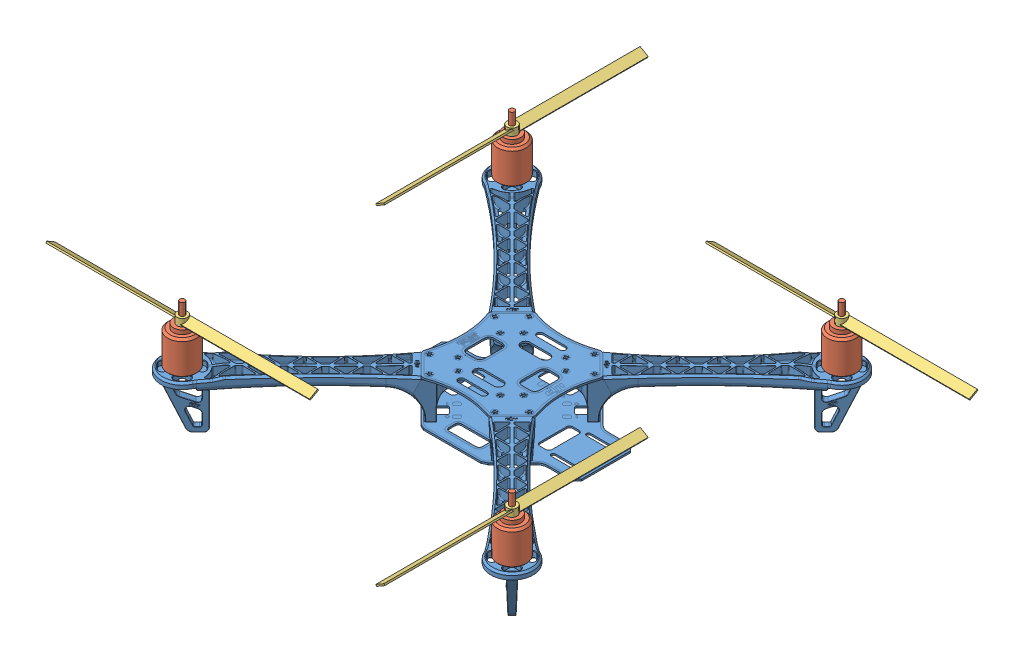
SolidWorks assembly 四旋翼机构, configuration 默认. Lengths in mm.
Overall size (571.82 108 571.82).
9 component instances, 3 part files, 26 mates.
Components (placement in the parent):
- F450 Quadcopter Frame-2: F450 Quadcopter Frame [默认] at (326.2395 -274.8713 170.1683) size (358.57 55.06 358.57)
- 旋翼电机改孔距-1: 旋翼电机改孔距 [默认] at (563.4779 -112.1783 79.5763) x (-1 0 0) z (0 0 -1) size (27.7 57 27.7)
- 螺旋桨-1: 螺旋桨 [默认] at (563.4779 -76.1783 79.5763) x (-1 0 0) z (0 0 -1) size (254 7 254)
- 旋翼电机改孔距-2: 旋翼电机改孔距 [默认] at (245.6651 -112.1783 79.5656) x (0 0 -1) z (1 0 0) size (27.7 57 27.7)
- 螺旋桨-2: 螺旋桨 [默认] at (245.6651 -76.1783 79.5656) x (0 0 -1) z (1 0 0) size (254 7 254)
- 旋翼电机改孔距-4: 旋翼电机改孔距 [默认] at (245.6757 -112.1783 -238.2473) size (27.7 57 27.7)
- 螺旋桨-4: 螺旋桨 [默认] at (245.6757 -76.1783 -238.2473) size (254 7 254)
- 旋翼电机改孔距-6: 旋翼电机改孔距 [默认] at (563.4886 -112.1783 -238.2366) x (0 0 1) z (-1 0 0) size (27.7 57 27.7)
- 螺旋桨-6: 螺旋桨 [默认] at (563.4886 -76.1783 -238.2366) x (0 0 1) z (-1 0 0) size (254 7 254)
Mates (geometry in assembly coordinates):
- 同心1: concentric: cylinder of 旋翼电机改孔距-1 through (563.4779 -57.6783 79.5763) axis (0 -1 0) radius 2.5; cylinder of 螺旋桨-1 through (563.4779 -76.1793 79.5763) axis (0 1 0) radius 2.5
- 重合1: coincident: plane of 旋翼电机改孔距-1 through (563.4779 -76.1783 79.5763) normal (0 1 0); plane of 螺旋桨-1 through (563.4779 -76.1783 79.5763) normal (0 -1 0)
- 重合2: coincident: plane of F450 Quadcopter Frame-2 through (570.6867 -112.1783 60.2935) normal (0 1 0); plane of 旋翼电机改孔距-1 through (563.4779 -112.1783 79.5763) normal (0 -1 0)
- 同心6: concentric: cylinder of F450 Quadcopter Frame-2 through (563.4779 -131.8204 79.5763) axis (0 1 0) radius 5; cylinder of 旋翼电机改孔距-1 through (563.4779 -114.6783 79.5763) axis (0 1 0) radius 2.5
- 同心9: concentric: cylinder of F450 Quadcopter Frame-2 through (554.1779 -131.8204 79.5763) axis (0 1 0) radius 1.65; cylinder of 旋翼电机改孔距-1 through (554.1779 -109.1783 79.5763) axis (0 -1 0) radius 1.35
- 同心10: concentric: cylinder of 旋翼电机改孔距-2 through (245.6651 -57.6783 79.5656) axis (0 -1 0) radius 2.5; cylinder of 螺旋桨-2 through (245.6651 -76.1793 79.5656) axis (0 1 0) radius 2.5
- 重合3: coincident: plane of 旋翼电机改孔距-2 through (245.6651 -76.1783 79.5656) normal (0 1 0); plane of 螺旋桨-2 through (245.6651 -76.1783 79.5656) normal (0 -1 0)
- 重合4: coincident: plane of F450 Quadcopter Frame-2 through (264.9479 -112.1783 86.7744) normal (0 1 0); plane of 旋翼电机改孔距-2 through (245.6651 -112.1783 79.5656) normal (0 -1 0)
- 同心11: concentric: cylinder of F450 Quadcopter Frame-2 through (245.6651 -131.8204 79.5656) axis (0 1 0) radius 5; cylinder of 旋翼电机改孔距-2 through (245.6651 -114.6783 79.5656) axis (0 1 0) radius 2.5
- 同心12: concentric: cylinder of F450 Quadcopter Frame-2 through (245.6651 -131.8204 70.2656) axis (0 1 0) radius 1.65; cylinder of 旋翼电机改孔距-2 through (245.6651 -109.1783 70.2656) axis (0 -1 0) radius 1.35
- 同心14: concentric: cylinder of 旋翼电机改孔距-4 through (245.6757 -57.6783 -238.2473) axis (0 -1 0) radius 2.5; cylinder of 螺旋桨-4 through (245.6757 -76.1793 -238.2473) axis (0 1 0) radius 2.5
- 重合6: coincident: plane of 旋翼电机改孔距-4 through (245.6757 -76.1783 -238.2473) normal (0 1 0); plane of 螺旋桨-4 through (245.6757 -76.1783 -238.2473) normal (0 -1 0)
- 重合7: coincident: plane of F450 Quadcopter Frame-2 through (238.4669 -112.1783 -218.9644) normal (0 1 0); plane of 旋翼电机改孔距-4 through (245.6757 -112.1783 -238.2473) normal (0 -1 0)
- 同心15: concentric: cylinder of F450 Quadcopter Frame-2 through (245.6757 -131.8204 -238.2473) axis (0 1 0) radius 5; cylinder of 旋翼电机改孔距-4 through (245.6757 -114.6783 -238.2473) axis (0 1 0) radius 2.5
- 同心16: concentric: cylinder of F450 Quadcopter Frame-2 through (254.9757 -131.8204 -238.2473) axis (0 1 0) radius 1.65; cylinder of 旋翼电机改孔距-4 through (254.9757 -109.1783 -238.2473) axis (0 -1 0) radius 1.35
- 同心18: concentric: cylinder of 旋翼电机改孔距-6 through (563.4886 -57.6783 -238.2366) axis (0 -1 0) radius 2.5; cylinder of 螺旋桨-6 through (563.4886 -76.1793 -238.2366) axis (0 1 0) radius 2.5
- 重合9: coincident: plane of 旋翼电机改孔距-6 through (563.4886 -76.1783 -238.2366) normal (0 1 0); plane of 螺旋桨-6 through (563.4886 -76.1783 -238.2366) normal (0 -1 0)
- 重合10: coincident: plane of F450 Quadcopter Frame-2 through (544.2058 -112.1783 -245.4454) normal (0 1 0); plane of 旋翼电机改孔距-6 through (563.4886 -112.1783 -238.2366) normal (0 -1 0)
- 同心19: concentric: cylinder of F450 Quadcopter Frame-2 through (563.4886 -131.8204 -238.2366) axis (0 1 0) radius 5; cylinder of 旋翼电机改孔距-6 through (563.4886 -114.6783 -238.2366) axis (0 1 0) radius 2.5
- 同心20: concentric: cylinder of F450 Quadcopter Frame-2 through (563.4886 -131.8204 -228.9366) axis (0 1 0) radius 1.65; cylinder of 旋翼电机改孔距-6 through (563.4886 -109.1783 -228.9366) axis (0 -1 0) radius 1.35
- 重合11: coincident: plane of F450 Quadcopter Frame-2 through (341.0768 -150.8283 -39.0874) normal (0 -1 0); plane of ? through (454.5768 -150.8283 -78.8984) normal (0 1 0)
- 同心21: concentric: cylinder of F450 Quadcopter Frame-2 through (461.7768 -150.8283 -61.8984) axis (0 1 0) radius 2; cylinder of ? through (461.7768 -160.8293 -61.8984) axis (0 1 0) radius 1.65
- 平行1: parallel: plane of F450 Quadcopter Frame-2 through (495.5768 -150.8283 -55.3984) normal (1 0 0); plane of ? through (479.5768 -150.8283 -101.3984) normal (1 0 0)
- 重合13: coincident: plane of F450 Quadcopter Frame-2 through (341.0768 -150.8283 -39.0874) normal (0 -1 0); plane of ? through (354.5768 -150.8283 -78.8984) normal (0 1 0)
- 同心22: concentric: cylinder of F450 Quadcopter Frame-2 through (347.3768 -150.8283 -95.8984) axis (0 1 0) radius 2; cylinder of ? through (347.3768 -160.8293 -95.8984) axis (0 1 0) radius 1.65
- 平行2: parallel: plane of F450 Quadcopter Frame-2 through (313.5768 -150.8283 -55.3984) normal (-1 0 0); plane of ? through (329.5768 -150.8283 -56.3984) normal (-1 0 0)
